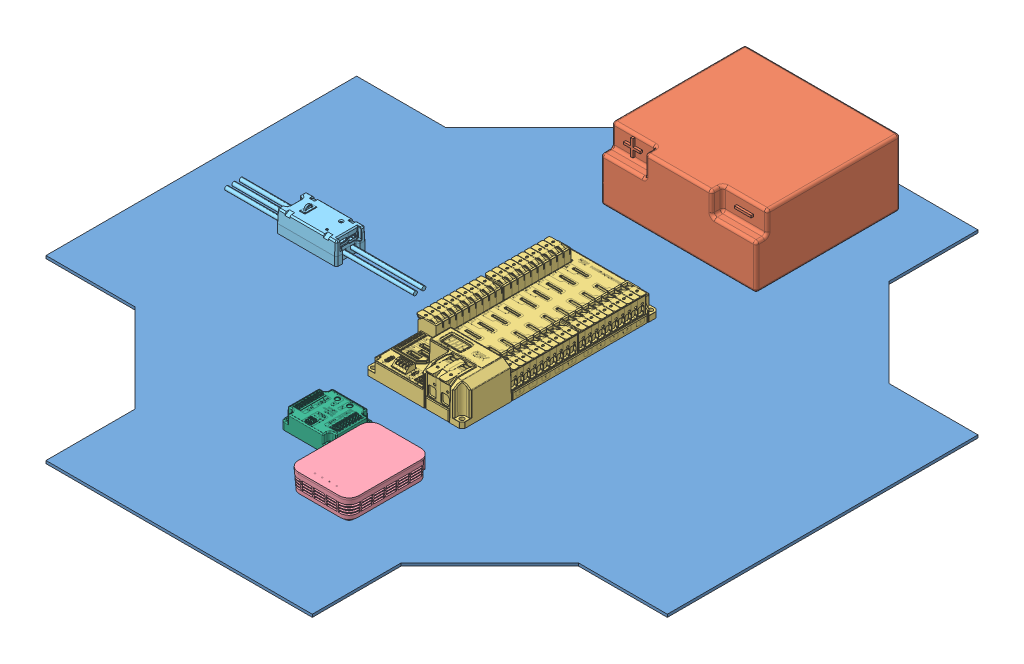
SolidWorks assembly 04-000 Belly Pan Electronics, configuration Default. Lengths in mm.
Overall size (711.2 79.38 762).
6 component instances, 6 part files, 10 mates.
Components (placement in the parent):
- 04-001 Belly Panel-1: 04-001 Belly Panel [Default] at origin size (711.2 3.17 762)
- Battery-1: Battery [Default] at (0 39.6875 -355.6) x (-1 0 0) z (0 1 0) size (177.8 165.1 76.2)
- Power Distribution Hub (REv-11-1850)-1: Power Distribution Hub (REv-11-1850) [Default] at (0 1.5875 0) size (112.73 39.72 227.13)
- OM5P-AC_Radio-1: OM5P-AC_Radio [Default] at (53.0318 5.3375 227.6264) size (69.52 26.25 94.01)
- SPARK MAX Motor Controller (REV-11-2158)-1: SPARK MAX Motor Controller (REV-11-2158) [Default] at (-211.7122 24.5375 6.6947) x (-1 0 0) z (0 0 1) size (152.48 29.65 34.5)
- Voltage Regulator Module (217-4245)-1: Voltage Regulator Module (217-4245) [Default] at (-21.2424 8.6935 187.1792) size (56.4 21.13 51.57)
Mates (geometry in assembly coordinates):
- Coincident1: coincident anti-aligned: plane of Battery-1 through (0 39.6875 -355.6) normal (-1 0 0)
- Coincident3: coincident anti-aligned: plane of 04-001 Belly Panel-1 through (0 1.5875 0) normal (0 1 0); plane of Battery-1 through (88.9 1.5875 -190.5) normal (0 -1 0)
- Distance1: distance = 25.4 mm aligned: plane of 04-001 Belly Panel-1 through (0 1.5875 -381) normal (0 0 -1); plane of Battery-1 through (0 39.6875 -355.6) normal (0 0 -1)
- Coincident5: coincident aligned: plane of Power Distribution Hub (REv-11-1850)-1 through (0 1.5875 0) normal (1 0 0)
- Coincident6: coincident anti-aligned: plane of 04-001 Belly Panel-1 through (0 1.5875 0) normal (0 1 0); plane of Power Distribution Hub (REv-11-1850)-1 through (-53.3407 1.5875 102.7728) normal (0 -1 0)
- Coincident8: coincident aligned: plane of Power Distribution Hub (REv-11-1850)-1 through (0 1.5875 0) normal (0 0 1)
- Coincident9: coincident anti-aligned: plane of 04-001 Belly Panel-1 through (0 1.5875 0) normal (0 1 0); plane of Voltage Regulator Module (217-4245)-1 through (2.1019 1.5875 167.632) normal (0 -1 0)
- Coincident10: coincident anti-aligned: plane of 04-001 Belly Panel-1 through (0 1.5875 0) normal (0 1 0); plane of OM5P-AC_Radio-1 through (53.0318 1.5875 227.6264) normal (0 -1 0)
- Coincident11: coincident anti-aligned: plane of 04-001 Belly Panel-1 through (0 1.5875 0) normal (0 1 0); plane of SPARK MAX Motor Controller (REV-11-2158)-1 through (-211.7122 1.5875 6.6947) normal (0 -1 0)
- Parallel2: parallel aligned: plane of 04-001 Belly Panel-1 through (0 1.5875 177.8) normal (0 0 1); plane of SPARK MAX Motor Controller (REV-11-2158)-1 through (-177.0872 12.0375 23.9447) normal (0 0 1)
